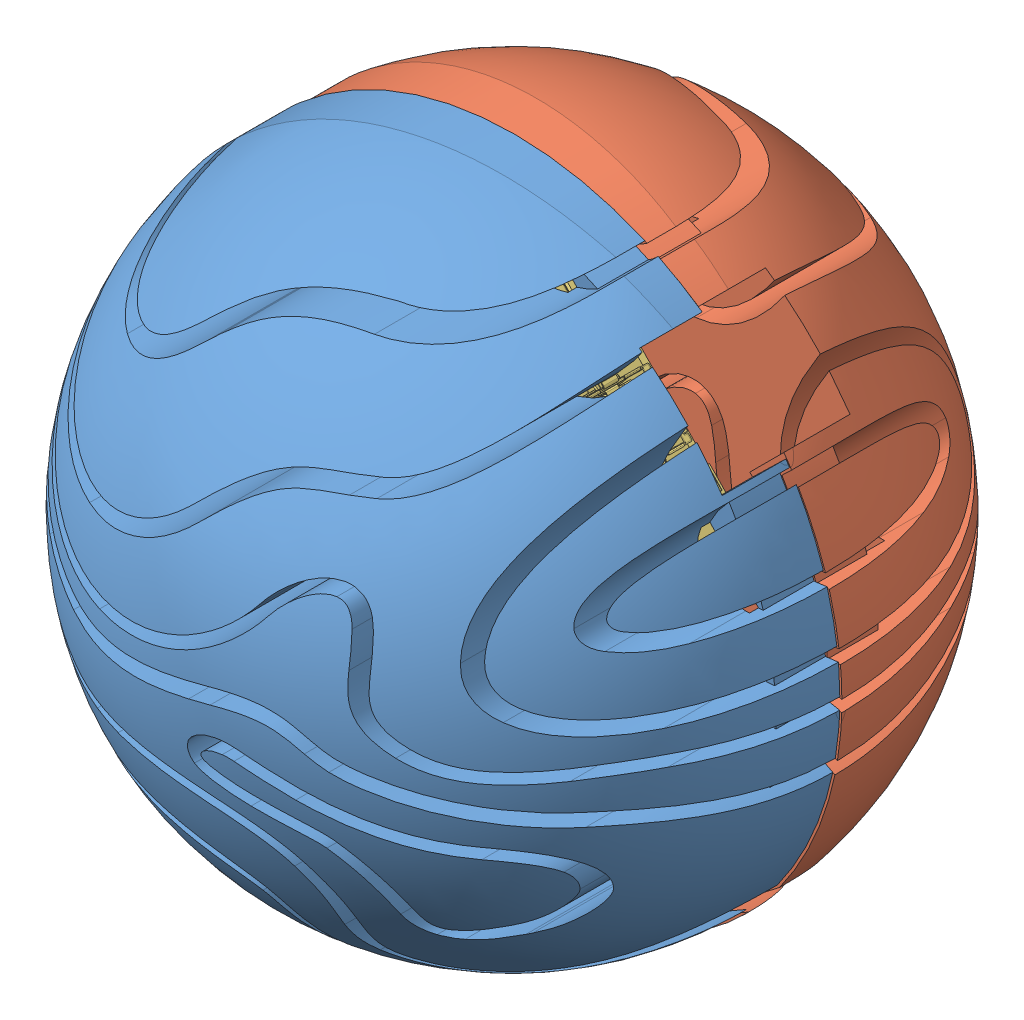
SolidWorks assembly Assem1, configuration Default. Lengths in mm.
Overall size (138.27 139.87 137.5).
3 component instances, 3 part files, 6 mates.
Components (placement in the parent):
- cosmo_boule_guirlande_male-1: cosmo_boule_guirlande_male [Default] at (-175.7638 -18.645 55.1316) size (137.84 139.62 83.75)
- cosmo_boule_guirlande_femelle-1: cosmo_boule_guirlande_femelle [Default] at (-175.2749 -18.8875 31.0795) size (137.84 139.62 72.66)
- Raspberry Pi 3-1: Raspberry Pi 3 [Default] at (-142.6896 12.9477 44.922) x (0.717279 0.696786 0) z (0 0 1) size (89.64 57.31 18.59)
Mates (geometry in assembly coordinates):
- Parallel1: parallel: plane of cosmo_boule_guirlande_male-1 through (-216.3415 -60.3107 61.112) normal (0 0 -1); plane of Raspberry Pi 3-1 through (-142.6896 12.9477 43.592) normal (0 0 -1)
- Parallel2: parallel: line of cosmo_boule_guirlande_male-1 through (-167.5179 -54.1144 48.612) axis (0.717279 0.696786 0); line of Raspberry Pi 3-1 through (-139.8632 58.0906 44.592) axis (-0.717279 -0.696786 0)
- Coincident8: coincident: plane of cosmo_boule_guirlande_male-1 through (-216.3415 -60.3107 61.112) normal (0 0 -1); line of Raspberry Pi 3-1 through (-146.7422 47.5593 61.112) axis (0.696786 -0.717279 0)
- Concentric1: concentric: cylinder of cosmo_boule_guirlande_male-1 through (-148.0489 -47.8843 33.612) axis (0 0 1) radius 7.5; cylinder of cosmo_boule_guirlande_femelle-1 through (-148.0489 -47.8843 39.237) axis (0 0 1) radius 8.125
- Concentric2: concentric: cylinder of cosmo_boule_guirlande_male-1 through (-204.2989 8.3657 33.612) axis (0 0 1) radius 7.5; cylinder of cosmo_boule_guirlande_femelle-1 through (-204.2989 8.3657 39.237) axis (0 0 1) radius 8.125
- Coincident9: coincident: plane of cosmo_boule_guirlande_male-1 through (-154.7348 -87.9062 48.612) normal (0 0 -1); plane of cosmo_boule_guirlande_femelle-1 through (-154.3012 -88.1582 48.612) normal (0 0 1)
